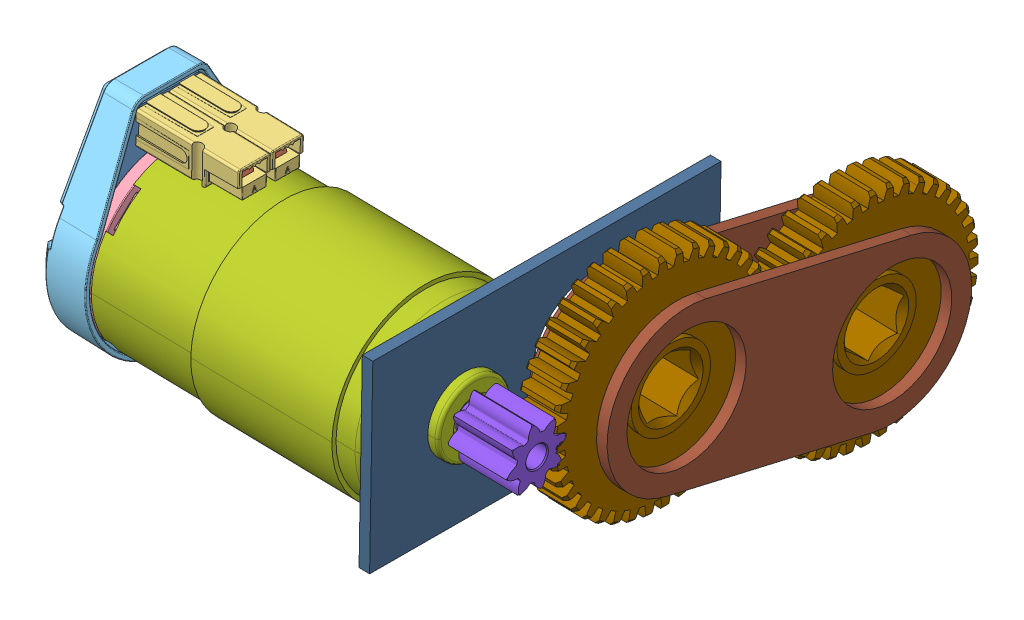
SolidWorks assembly Wrist Motion Test, configuration Default. Lengths in mm.
Overall size (104.18 83.46 140.06).
22 component instances, 11 part files, 17 mates.
Components (placement in the parent):
- 775pro (775pro Connect and 8T Pinion) (217-6459)-1: 775pro (775pro Connect and 8T Pinion) (217-6459) [Default] at (-150.4553 -33.8495 58.3455) x (0.002773 0 -0.999996) z (0.999844 -0.017452 0.002772) size (44.99 55.15 97.74)
  - 775pro (775pro Connect and 8T Pinion) (217-6459)(2)^775pro (775pro Connect and 8T Pinion) (217-6459)-1: 775pro (775pro Connect and 8T Pinion) (217-6459)(2)^775pro (775pro Connect and 8T Pinion) (217-6459) [Default] at origin size (44.99 55.15 97.74) (virtual)
    - 217-6457-000 Rev2^775pro (775pro Connect and 8T Pinion) (217-6459)(2)_775pro (775pro Connect and 8T Pinion) (217-6459)-1: 217-6457-000 Rev2^775pro (775pro Connect and 8T Pinion) (217-6459)(2)_775pro (775pro Connect and 8T Pinion) (217-6459) [Default] at (0 0 -66.1) x (1 0 0) z (0 1 0) size (44.99 33.26 55.15) (virtual)
      - 217-6457-900 Rev1^217-6457-000 Rev2_775pro (775pro Connect and 8T Pinion) (217-6459)(2)_775pro (775pro Connect and 8T Pinion) (217-6459)-1: 217-6457-900 Rev1^217-6457-000 Rev2_775pro (775pro Connect and 8T Pinion) (217-6459)(2)_775pro (775pro Connect and 8T Pinion) (217-6459) [Default] at (0 5.3622 0) x (-1 0 0.000693) z (0.000693 0 1) size (41.5 28.13 51.51) (virtual)
        - 217-6457-901 Rev3_Instruction Config^217-6457-900 Rev1_217-6457-000 Rev2_775pro (775pro Connect and 8T Pinion) (217-6459)(2)_775pro (775pro Connect and 8T Pinion) (217-6459)-1: 217-6457-901 Rev3_Instruction Config^217-6457-900 Rev1_217-6457-000 Rev2_775pro (775pro Connect and 8T Pinion) (217-6459)(2)_775pro (775pro Connect and 8T Pinion) (217-6459) [Default] at origin size (41.5 2.36 51.5) (virtual)
        - 30-45BBS Rev1_SHORTENED CONTACT^217-6457-900 Rev1_217-6457-000 Rev2_775pro (775pro Connect and 8T Pinion) (217-6459)(2)_775pro (775pro Connect and 8T Pinion) (217-6459)-1: 30-45BBS Rev1_SHORTENED CONTACT^217-6457-900 Rev1_217-6457-000 Rev2_775pro (775pro Connect and 8T Pinion) (217-6459)(2)_775pro (775pro Connect and 8T Pinion) (217-6459) [Default] at (3.95 14.4494 26.711) x (0 1 0) z (0 0 -1) size (26 3.6 2) (virtual)
        - 30-45BBS Rev1_SHORTENED CONTACT^217-6457-900 Rev1_217-6457-000 Rev2_775pro (775pro Connect and 8T Pinion) (217-6459)(2)_775pro (775pro Connect and 8T Pinion) (217-6459)-2: 30-45BBS Rev1_SHORTENED CONTACT^217-6457-900 Rev1_217-6457-000 Rev2_775pro (775pro Connect and 8T Pinion) (217-6459)(2)_775pro (775pro Connect and 8T Pinion) (217-6459) [Default] at (-3.9748 14.4494 26.711) x (0 1 0) z (0 0 -1) size (26 3.6 2) (virtual)
        - PA45XX-X Rev1^217-6457-900 Rev1_217-6457-000 Rev2_775pro (775pro Connect and 8T Pinion) (217-6459)(2)_775pro (775pro Connect and 8T Pinion) (217-6459)-1: PA45XX-X Rev1^217-6457-900 Rev1_217-6457-000 Rev2_775pro (775pro Connect and 8T Pinion) (217-6459)(2)_775pro (775pro Connect and 8T Pinion) (217-6459) [Default] at (-8.4198 2.3622 73.1531) x (0 1 0) z (-1 0 0) size (24.71 8.41 8.41) (virtual)
        - PA45XX-X Rev1^217-6457-900 Rev1_217-6457-000 Rev2_775pro (775pro Connect and 8T Pinion) (217-6459)(2)_775pro (775pro Connect and 8T Pinion) (217-6459)-2: PA45XX-X Rev1^217-6457-900 Rev1_217-6457-000 Rev2_775pro (775pro Connect and 8T Pinion) (217-6459)(2)_775pro (775pro Connect and 8T Pinion) (217-6459) [Default] at (-0.495 2.3622 73.1531) x (0 1 0) z (-1 0 0) size (24.71 8.41 8.41) (virtual)
      - 217-6457-001 Rev4^217-6457-000 Rev2_775pro (775pro Connect and 8T Pinion) (217-6459)(2)_775pro (775pro Connect and 8T Pinion) (217-6459)-1: 217-6457-001 Rev4^217-6457-000 Rev2_775pro (775pro Connect and 8T Pinion) (217-6459)(2)_775pro (775pro Connect and 8T Pinion) (217-6459) [Default] at origin size (41.49 7.8 41.49) (virtual)
      - 217-6457-002 Rev7^217-6457-000 Rev2_775pro (775pro Connect and 8T Pinion) (217-6459)(2)_775pro (775pro Connect and 8T Pinion) (217-6459)-1: 217-6457-002 Rev7^217-6457-000 Rev2_775pro (775pro Connect and 8T Pinion) (217-6459)(2)_775pro (775pro Connect and 8T Pinion) (217-6459) [Default] at (0 0.05 0) size (44.99 11.5 55.15) (virtual)
      - 217-9191-008 Rev1^217-6457-000 Rev2_775pro (775pro Connect and 8T Pinion) (217-6459)(2)_775pro (775pro Connect and 8T Pinion) (217-6459)-1: 217-9191-008 Rev1^217-6457-000 Rev2_775pro (775pro Connect and 8T Pinion) (217-6459)(2)_775pro (775pro Connect and 8T Pinion) (217-6459) [Default] at (81.4247 7.8 32.3804) x (-0.560945 0 -0.827853) z (0 1 0) size (4.2 4.2 11.81) (virtual)
      - 217-9191-008 Rev1^217-6457-000 Rev2_775pro (775pro Connect and 8T Pinion) (217-6459)(2)_775pro (775pro Connect and 8T Pinion) (217-6459)-2: 217-9191-008 Rev1^217-6457-000 Rev2_775pro (775pro Connect and 8T Pinion) (217-6459)(2)_775pro (775pro Connect and 8T Pinion) (217-6459) [Default] at (32.3804 7.8 -81.4247) x (-0.827853 0 0.560945) z (0 1 0) size (4.2 4.2 11.81) (virtual)
      - 217-9191-008 Rev1^217-6457-000 Rev2_775pro (775pro Connect and 8T Pinion) (217-6459)(2)_775pro (775pro Connect and 8T Pinion) (217-6459)-3: 217-9191-008 Rev1^217-6457-000 Rev2_775pro (775pro Connect and 8T Pinion) (217-6459)(2)_775pro (775pro Connect and 8T Pinion) (217-6459) [Default] at (-81.4247 7.8 -32.3804) x (0.560945 0 0.827853) z (0 1 0) size (4.2 4.2 11.81) (virtual)
      - 217-9191-008 Rev1^217-6457-000 Rev2_775pro (775pro Connect and 8T Pinion) (217-6459)(2)_775pro (775pro Connect and 8T Pinion) (217-6459)-4: 217-9191-008 Rev1^217-6457-000 Rev2_775pro (775pro Connect and 8T Pinion) (217-6459)(2)_775pro (775pro Connect and 8T Pinion) (217-6459) [Default] at (-32.3804 7.8 81.4247) x (0.827853 0 -0.560945) z (0 1 0) size (4.2 4.2 11.81) (virtual)
    - 217-4347-000 Rev2^775pro (775pro Connect and 8T Pinion) (217-6459)(2)_775pro (775pro Connect and 8T Pinion) (217-6459)-1: 217-4347-000 Rev2^775pro (775pro Connect and 8T Pinion) (217-6459)(2)_775pro (775pro Connect and 8T Pinion) (217-6459) [Default] x (0 0 -1) z (1 0 0) size (88 44.3 44.3) (virtual)
    - 217-6362-001 Rev2_Spur01^775pro (775pro Connect and 8T Pinion) (217-6459)(2)_775pro (775pro Connect and 8T Pinion) (217-6459)-1: 217-6362-001 Rev2_Spur01^775pro (775pro Connect and 8T Pinion) (217-6459)(2)_775pro (775pro Connect and 8T Pinion) (217-6459) [Default] at (0 0 12.9437) x (0.84924 0.528008 0) z (0 0 1) size (13.62 13.62 16.29) (virtual)
- am-4710 40T 20DP 500hex 375 FW-1: am-4710 40T 20DP 500hex 375 FW [Default] at (-139.81 -34.0338 27.8949) x (0.999844 -0.017452 0.002772) z (0.016108 0.964608 0.263196) size (12.7 53.24 53.24)
- Part15^Wrist Motion Test-1: Part15^Wrist Motion Test [Default] at (-150.4553 -33.8495 58.3455) x (0.002773 0 -0.999996) z (0.999844 -0.017452 0.002772) size (83.45 44.65 2.54) (virtual)
- am-4710 40T 20DP 500hex 375 FW-2: am-4710 40T 20DP 500hex 375 FW [Default] at (-139.8738 -45.5476 -21.583) x (0.999844 -0.017452 0.002772) z (0.009458 0.661023 0.750306) size (12.7 53.24 53.24)
- Part16^Wrist Motion Test-1: Part16^Wrist Motion Test [Default] at (-141.3972 -34.0061 27.8905) x (0.017407 0.999725 0.01574) z (-0.999844 0.017452 -0.002772) size (50.39 87.39 2.54) (virtual)
- Part16^Wrist Motion Test-2: Part16^Wrist Motion Test [Default] at (-124.9104 -34.2939 27.9362) x (0.017407 0.999725 0.01574) z (-0.999844 0.017452 -0.002772) size (50.39 87.39 2.54) (virtual)
Mates (geometry in assembly coordinates):
- Parallel1: parallel anti-aligned: plane of 775pro (775pro Connect and 8T Pinion) (217-6459)-1/775pro (775pro Connect and 8T Pinion) (217-6459)(2)^775pro (775pro Connect and 8T Pinion) (217-6459)-1/217-6362-001 Rev2_Spur01^775pro (775pro Connect and 8T Pinion) (217-6459)(2)_775pro (775pro Connect and 8T Pinion) (217-6459)-1 through (-130.371 -34.2001 58.4012) normal (0.999844 -0.017452 0.002772); plane of am-4710 40T 20DP 500hex 375 FW-1 through (-139.81 -34.0338 27.8949) normal (-0.999844 0.017452 -0.002772)
- GearMate1: gear = 1016 : 203.2 mm: cylinder of 775pro (775pro Connect and 8T Pinion) (217-6459)-1/775pro (775pro Connect and 8T Pinion) (217-6459)(2)^775pro (775pro Connect and 8T Pinion) (217-6459)-1/217-6362-001 Rev2_Spur01^775pro (775pro Connect and 8T Pinion) (217-6459)(2)_775pro (775pro Connect and 8T Pinion) (217-6459)-1 through (-130.371 -34.2001 58.4012) axis (-0.999844 0.017452 -0.002772) radius 2.48; cylinder of am-4710 40T 20DP 500hex 375 FW-1 through (-128.6992 -34.2278 27.9257) axis (-0.999844 0.017452 -0.002772) radius 9.525
- Coincident4: coincident aligned: plane of 775pro (775pro Connect and 8T Pinion) (217-6459)-1/775pro (775pro Connect and 8T Pinion) (217-6459)(2)^775pro (775pro Connect and 8T Pinion) (217-6459)-1/217-6362-001 Rev2_Spur01^775pro (775pro Connect and 8T Pinion) (217-6459)(2)_775pro (775pro Connect and 8T Pinion) (217-6459)-1 through (-130.371 -34.2001 58.4012) normal (0.999844 -0.017452 0.002772); plane of am-4710 40T 20DP 500hex 375 FW-1 through (-130.2865 -34.2001 27.9213) normal (0.999844 -0.017452 0.002772)
- InPlace1: in place: plane of ? through (-136.6852 55.8423 67.0864) normal (1 0 0); plane of ? through (-136.6852 0 0) normal (1 0 0); moOrthogonalPlaneRef_w of ? through (-136.6852 55.8423 67.0864) normal (1 0 0); plane of ? through (-136.6852 0 0) normal (0 1 0); plane of ? through (-136.6852 55.8423 67.0864) normal (1 0 0); plane of ? through (-136.6852 0 0) normal (0 0 -1); plane of 775pro (775pro Connect and 8T Pinion) (217-6459)-1/775pro (775pro Connect and 8T Pinion) (217-6459)(2)^775pro (775pro Connect and 8T Pinion) (217-6459)-1/217-4347-000 Rev2^775pro (775pro Connect and 8T Pinion) (217-6459)(2)_775pro (775pro Connect and 8T Pinion) (217-6459)-1 through (-150.3026 -25.1008 58.3459) normal (0.999844 -0.017452 0.002772); unknown of Part15^Wrist Motion Test-1
- Coincident5: coincident aligned: plane of 775pro (775pro Connect and 8T Pinion) (217-6459)-1/775pro (775pro Connect and 8T Pinion) (217-6459)(2)^775pro (775pro Connect and 8T Pinion) (217-6459)-1/217-4347-000 Rev2^775pro (775pro Connect and 8T Pinion) (217-6459)(2)_775pro (775pro Connect and 8T Pinion) (217-6459)-1; plane of Part15^Wrist Motion Test-1
- Coincident6: coincident aligned: moOrthogonalPlaneRef_w of 775pro (775pro Connect and 8T Pinion) (217-6459)-1/775pro (775pro Connect and 8T Pinion) (217-6459)(2)^775pro (775pro Connect and 8T Pinion) (217-6459)-1/217-4347-000 Rev2^775pro (775pro Connect and 8T Pinion) (217-6459)(2)_775pro (775pro Connect and 8T Pinion) (217-6459)-1; plane of Part15^Assem5-1 through (-150.4553 -33.8495 58.3455) normal (0.017452 0.999848 0.000048)
- Coincident7: coincident anti-aligned: moOrthogonalPlaneRef_w of 775pro (775pro Connect and 8T Pinion) (217-6459)-1/775pro (775pro Connect and 8T Pinion) (217-6459)(2)^775pro (775pro Connect and 8T Pinion) (217-6459)-1/217-4347-000 Rev2^775pro (775pro Connect and 8T Pinion) (217-6459)(2)_775pro (775pro Connect and 8T Pinion) (217-6459)-1; plane of Part15^Assem5-1 through (-150.4553 -33.8495 58.3455) normal (0.002773 0 -0.999996)
- Coincident8: coincident aligned: plane of 775pro (775pro Connect and 8T Pinion) (217-6459)-1/775pro (775pro Connect and 8T Pinion) (217-6459)(2)^775pro (775pro Connect and 8T Pinion) (217-6459)-1/217-6457-000 Rev2^775pro (775pro Connect and 8T Pinion) (217-6459)(2)_775pro (775pro Connect and 8T Pinion) (217-6459)-1/217-6457-002 Rev7^217-6457-000 Rev2_775pro (775pro Connect and 8T Pinion) (217-6459)(2)_775pro (775pro Connect and 8T Pinion) (217-6459)-1 through (-216.0423 0 64.6337) normal (0 1 0)
- Coincident10: coincident aligned: plane of am-4710 40T 20DP 500hex 375 FW-1 through (-130.2865 -34.2001 27.9213) normal (0.999844 -0.017452 0.002772); plane of am-4710 40T 20DP 500hex 375 FW-2 through (-130.3502 -45.7138 -21.5566) normal (0.999844 -0.017452 0.002772)
- GearMate2: gear = 19.05 : 19.05 mm: cylinder of am-4710 40T 20DP 500hex 375 FW-1 through (-128.6992 -34.2278 27.9257) axis (-0.999844 0.017452 -0.002772) radius 9.525; cylinder of am-4710 40T 20DP 500hex 375 FW-2 through (-128.763 -45.7415 -21.5522) axis (-0.999844 0.017452 -0.002772) radius 9.525
- Parallel2: parallel aligned: cylinder of am-4710 40T 20DP 500hex 375 FW-1 through (-128.6992 -34.2278 27.9257) axis (-0.999844 0.017452 -0.002772) radius 9.525; cylinder of am-4710 40T 20DP 500hex 375 FW-2 through (-128.763 -45.7415 -21.5522) axis (-0.999844 0.017452 -0.002772) radius 9.525
- Concentric4: concentric aligned: cylinder of am-4710 40T 20DP 500hex 375 FW-1 through (-128.6992 -34.2278 27.9257) axis (-0.999844 0.017452 -0.002772) radius 9.525; cylinder of Part15^Wrist Motion Test-1 through (-147.8312 -33.8938 27.8727) axis (-0.999844 0.017452 -0.002772) radius 14.2875
- Concentric5: concentric anti-aligned: cylinder of Part15^Wrist Motion Test-1 through (-147.8312 -33.8938 27.8727) axis (-0.999844 0.017452 -0.002772) radius 14.2875; cylinder of Part16^Wrist Motion Test-1 through (-143.9368 -33.9618 27.8835) axis (0.999844 -0.017452 0.002772) radius 14.2875
- Concentric8: concentric aligned: cylinder of am-4710 40T 20DP 500hex 375 FW-2 through (-141.461 -45.5199 -21.5875) axis (0.999844 -0.017452 0.002772) radius 9.525; cylinder of Part16^Wrist Motion Test-1 through (-144.0006 -45.4756 -21.5945) axis (0.999844 -0.017452 0.002772) radius 14.2875
- Coincident11: coincident anti-aligned: plane of am-4710 40T 20DP 500hex 375 FW-2 through (-141.461 -45.5199 -21.5875) normal (-0.999844 0.017452 -0.002772); plane of Part16^Wrist Motion Test-1 through (-141.3972 -34.0061 27.8905) normal (0.999844 -0.017452 0.002772)
- Concentric9: concentric anti-aligned: cylinder of am-4710 40T 20DP 500hex 375 FW-1 through (-128.6992 -34.2278 27.9257) axis (-0.999844 0.017452 -0.002772) radius 9.525; cylinder of Part16^Wrist Motion Test-2 through (-127.45 -34.2496 27.9292) axis (0.999844 -0.017452 0.002772) radius 14.2875
- Concentric10: concentric anti-aligned: cylinder of am-4710 40T 20DP 500hex 375 FW-2 through (-128.763 -45.7415 -21.5522) axis (-0.999844 0.017452 -0.002772) radius 9.525; cylinder of Part16^Wrist Motion Test-2 through (-127.5137 -45.7633 -21.5488) axis (0.999844 -0.017452 0.002772) radius 14.2875
